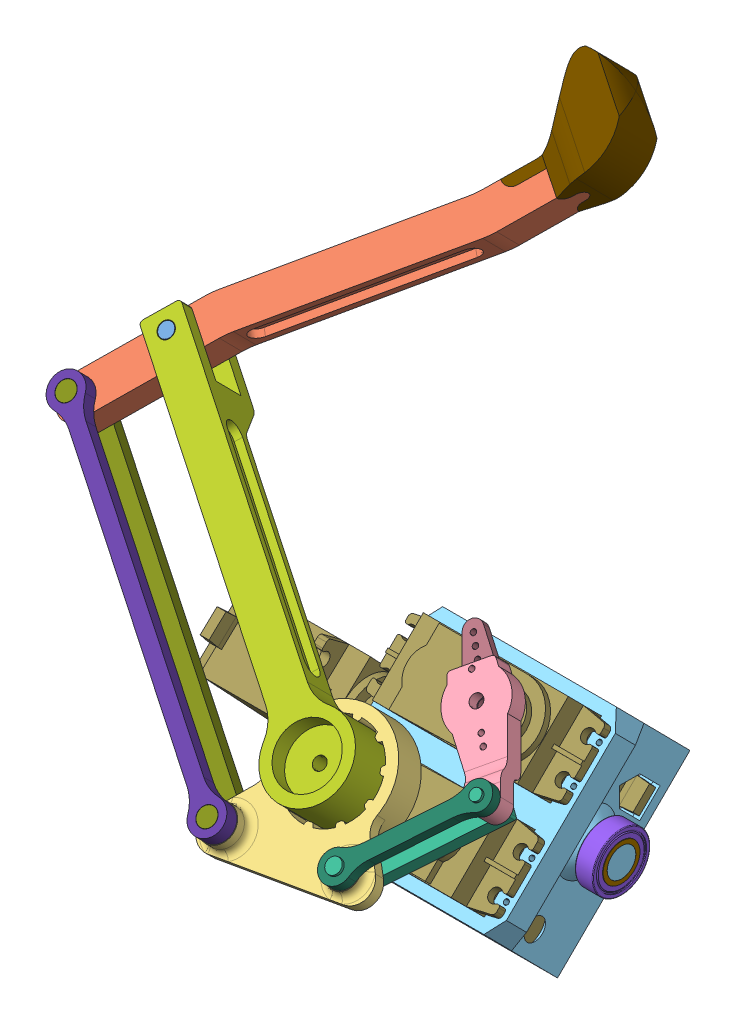
SolidWorks assembly Leg 2, configuration Default. Lengths in mm.
Overall size (147.89 165.46 140.11).
31 component instances, 18 part files, 42 mates.
Components (placement in the parent):
- Dowel-1: Dowel [Default] at (-255.223 372.999 -15.2268) x (0.218857 -0.685853 0.694051) z (0 0.711295 0.702894) size (3.9 3.9 20)
- Lower leg-1: Lower leg [Default] at (-184.6898 434.9539 -55.8705) x (0.812101 -0.41015 0.415052) z (0 -0.711295 -0.702894) size (20 126 9)
- Rotating Piece-1: Rotating Piece [Default] at (-173.9415 332.1367 27.2621) x (0.180878 0.6913 -0.699562) z (0.983506 -0.127138 0.128657) size (44.28 13.7 43.21)
- Servo Arm Mount-1: Servo Arm Mount [Default] at (-152.9415 354.3242 12.3496) x (-0.715783 -0.490847 0.496713) z (0 0.711295 0.702894) size (16.2 34.39 8.1)
- Servo Housing 3-1: Servo Housing 3 [Default] at (-163.4415 323.5657 18.6498) x (1 0 0) z (0 0.711295 0.702894) size (61.5 52 29.25)
- Short Connecting Rod-1: Short Connecting Rod [Default] at (-137.7959 345.0213 22.475) x (-0.625384 -0.54848 0.555035) z (0 -0.711295 -0.702894) size (37.08 4 13)
- Upper Leg-1: Upper Leg [Default] at (-261.8797 379.1638 -7.2384) x (-0.587065 -0.569021 0.575822) z (0 0.711295 0.702894) size (22 116.4 18)
- 688ZZ Bearing Assembly-1: 688ZZ Bearing Assembly [Default] at (-131.6915 320.8602 -2.3002) x (0 0 -1) z (1 0 0) size (17.99 17.98 5)
  - Outer Ring-1: Outer Ring [Default] at origin size (16 16 5)
  - Inner Ring-1: Inner Ring [Default] x (-0.241565 -0.970385 0) z (0 0 1) size (10.6 10.6 5)
  - Cage-1: Cage [Default] x (0.535517 0.844524 0) z (0 0 1) size (13.01 13.06 2.21)
  - 2mm Ball Bearing-1: 2mm Ball Bearing [Default] at (-5.0671 3.2131 0) x (0.050652 0.835774 0.546732) z (0.977207 -0.154478 0.145614) size (2 2 2)
  - 2mm Ball Bearing-2: 2mm Ball Bearing [Default] at (-5.988 -0.3789 0) x (-0.450278 0.705928 0.546732) z (0.881377 0.449412 0.145614) size (2 2 2)
  - 2mm Ball Bearing-3: 2mm Ball Bearing [Default] at (-4.6217 -3.8262 0) x (-0.779216 0.306441 0.546732) z (0.448891 0.881642 0.145614) size (2 2 2)
  - 2mm Ball Bearing-4: 2mm Ball Bearing [Default] at (-1.49 -5.812 0) x (-0.810521 -0.210096 0.546732) z (-0.155056 0.977115 0.145614) size (2 2 2)
  - 2mm Ball Bearing-5: 2mm Ball Bearing [Default] at (2.2108 -5.5778 0) x (-0.532234 -0.646383 0.546732) z (-0.699777 0.699363 0.145614) size (2 2 2)
  - 2mm Ball Bearing-6: 2mm Ball Bearing [Default] at (5.0671 -3.2131 0) x (-0.050652 -0.835774 0.546732) z (-0.977207 0.154478 0.145614) size (2 2 2)
  - 2mm Ball Bearing-7: 2mm Ball Bearing [Default] at (5.988 0.3789 0) x (0.450278 -0.705928 0.546732) z (-0.881377 -0.449412 0.145614) size (2 2 2)
  - 2mm Ball Bearing-8: 2mm Ball Bearing [Default] at (4.6217 3.8262 0) x (0.779216 -0.306441 0.546732) z (-0.448891 -0.881642 0.145614) size (2 2 2)
  - 2mm Ball Bearing-9: 2mm Ball Bearing [Default] at (1.49 5.812 0) x (0.810521 0.210096 0.546732) z (0.155056 -0.977115 0.145614) size (2 2 2)
  - 2mm Ball Bearing-10: 2mm Ball Bearing [Default] at (-2.2108 5.5778 0) x (0.532234 0.646383 0.546732) z (0.699777 -0.699363 0.145614) size (2 2 2)
- MG996R-1: MG996R [Default] at (-163.4415 321.9958 -19.4546) x (-1 0 0) z (0 0.702894 -0.711295) size (54.5 42.75 20)
- MG996R-2: MG996R [Default] at (-163.4415 303.7205 -0.9609) x (1 0 0) z (0 -0.702894 0.711295) size (54.5 42.75 20)
- Double_Blade_Rudder-1: Double_Blade_Rudder [默认] at (-152.9415 354.2531 12.2793) x (-0.715783 -0.490847 0.496713) z (0.698322 -0.50312 0.509133) size (12.2 5.5 38)
- Circle Rudder-2: Circle Rudder [默认] at (-173.9415 335.8354 30.9171) x (0.268347 0.677113 -0.685206) z (-0.963322 0.18862 -0.190874) size (20.8 5.5 20.8)
- Circle Rudder-3: Circle Rudder [默认] at (-190.6915 320.8602 -2.3002) x (0 0.990513 -0.137416) z (0 0.137416 0.990513) size (20.8 5.5 20.8)
- MG996R-3: MG996R [Default] at (-235.7415 313.2801 -9.5667) x (0 -0.728522 -0.685022) z (0 -0.685022 0.728522) size (54.5 42.75 20)
- Short Connecting Rod Alt-1: Short Connecting Rod Alt [Default] at (-158.1737 328.6713 46.5607) x (-0.625384 -0.54848 0.555035) z (-0.780317 0.439579 -0.444832) size (41.18 3 8.1)
- Long Connecting Rod-1: Long Connecting Rod [Default] at (-185.0416 322.3134 45.3121) x (0.80954 -0.412644 0.417576) z (0 -0.711295 -0.702894) size (105.4 5 16)
- Long Connecting Rod Alt-1: Long Connecting Rod Alt [Default] at (-188.5331 327.6128 51.3309) x (0.80954 -0.412644 0.417576) z (-0.587065 -0.569021 0.575821) size (109.5 4 9.1)
- Foot Cap R2-1: Foot Cap R2 [Default] at (-184.6898 434.9539 -55.8705) x (0.812101 -0.41015 0.415052) z (0 -0.711295 -0.702894) size (26.22 31.5 15)
Mates (geometry in assembly coordinates):
- Coincident1: coincident anti-aligned: plane of Servo Housing 3-1 through (-163.4415 260.0708 -66.5893) normal (0 0.702894 -0.711295); plane of MG996R-1 through (-143.1915 340.3956 12.7868) normal (0 -0.702894 0.711295)
- Concentric1: concentric aligned: cylinder of Servo Housing 3-1 through (-138.4415 331.0182 -3.83) axis (0 0.711295 0.702894) radius 0.7; cylinder of MG996R-1 through (-138.4415 338.0245 3.0935) axis (0 0.711295 0.702894) radius 1.7678
- Distance1: distance = 1.85 mm anti-aligned: plane of MG996R-1 through (-138.4415 338.0245 3.0935) normal (0 -0.711295 -0.702894); plane of Servo Housing 3-1 through (-163.4415 321.7874 16.8926) normal (0 0.711295 0.702894)
- Coincident6: coincident aligned: plane of MG996R-1 through (-138.4415 339.8027 4.8507) normal (0 0.711295 0.702894); plane of MG996R-2 through (-188.4415 328.2356 16.556) normal (0 0.711295 0.702894)
- Concentric7: concentric aligned: cylinder of MG996R-1 through (-152.9415 350.341 8.4134) axis (0 0.711295 0.702894) radius 1.5; cylinder of Double_Blade_Rudder-1 through (-152.9415 350.341 8.4134) axis (0 0.711295 0.702894) radius 3
- Concentric8: concentric aligned: cylinder of MG996R-2 through (-173.9415 331.9233 27.0512) axis (0 0.711295 0.702894) radius 1.5; cylinder of Circle Rudder-2 through (-173.9415 331.9233 27.0512) axis (0 0.711295 0.702894) radius 3
- Coincident8: coincident anti-aligned: plane of MG996R-2 through (-173.9415 331.9233 27.0512) normal (0 0.711295 0.702894); plane of Circle Rudder-2 through (-173.9415 331.9233 27.0512) normal (0 -0.711295 -0.702894)
- Coincident9: coincident anti-aligned: plane of MG996R-1 through (-152.9415 350.341 8.4134) normal (0 0.711295 0.702894); plane of Double_Blade_Rudder-1 through (-152.9415 350.341 8.4134) normal (0 -0.711295 -0.702894)
- Coincident10: coincident anti-aligned: plane of Servo Housing 3-1 through (-190.6915 248.8245 -55.2086) normal (-1 0 0); plane of Circle Rudder-3 through (-190.6915 320.8602 -2.3002) normal (1 0 0)
- Concentric9: concentric anti-aligned: cylinder of Servo Housing 3-1 through (-170.6915 320.8602 -2.3002) axis (-1 0 0) radius 4.5; cylinder of Circle Rudder-3 through (-196.1915 320.8602 -2.3002) axis (1 0 0) radius 3
- Concentric10: concentric anti-aligned: cylinder of Servo Arm Mount-1 through (-152.9415 356.4581 14.4583) axis (0 -0.711295 -0.702894) radius 1.7; cylinder of Double_Blade_Rudder-1 through (-152.9415 352.6171 10.6626) axis (0 0.711295 0.702894) radius 1.5
- Coincident11: coincident anti-aligned: plane of Servo Arm Mount-1 through (-152.9415 354.2531 12.2793) normal (0 -0.711295 -0.702894); plane of Double_Blade_Rudder-1 through (-152.9415 354.2531 12.2793) normal (0 0.711295 0.702894)
- Concentric11: concentric aligned: cylinder of Servo Arm Mount-1 through (-145.9582 349.2219 17.3706) axis (0 0.711295 0.702894) radius 0.75; cylinder of Double_Blade_Rudder-1 through (-145.9582 347.5859 15.754) axis (0 0.711295 0.702894) radius 0.75
- Concentric12: concentric anti-aligned: cylinder of Servo Housing 3-1 through (-129.1915 320.8602 -2.3002) axis (-1 0 0) radius 4; cylinder of 688ZZ Bearing Assembly-1/Inner Ring-1 through (-124.9361 320.8602 -2.3002) axis (1 0 0) radius 4
- Coincident12: coincident anti-aligned: plane of Servo Housing 3-1 through (-134.1915 320.8602 -2.3002) normal (1 0 0); plane of 688ZZ Bearing Assembly-1/Inner Ring-1 through (-134.1915 319.6162 -7.2977) normal (-1 0 0)
- Coincident13: coincident anti-aligned: plane of Upper Leg-1 through (-173.9415 335.8354 30.9171) normal (0 -0.711295 -0.702894); plane of Circle Rudder-2 through (-173.9415 335.8354 30.9171) normal (0 0.711295 0.702894)
- Concentric13: concentric anti-aligned: cylinder of Upper Leg-1 through (-173.9415 342.237 37.2431) axis (0 -0.711295 -0.702894) radius 1.7; cylinder of Circle Rudder-2 through (-173.9415 334.1994 29.3004) axis (0 0.711295 0.702894) radius 1.5
- Concentric14: concentric aligned: cylinder of Servo Housing 3-1 through (-188.4415 312.4222 14.9882) axis (0 0.711295 0.702894) radius 0.7; cylinder of MG996R-2 through (-188.4415 319.4285 21.9117) axis (0 0.711295 0.702894) radius 1.7678
- Concentric15: concentric aligned: cylinder of Servo Housing 3-1 through (-188.4415 319.4512 7.8753) axis (0 0.711295 0.702894) radius 0.7; cylinder of MG996R-2 through (-188.4415 326.4574 14.7988) axis (0 0.711295 0.702894) radius 1.7678
- Concentric16: concentric anti-aligned: cylinder of Rotating Piece-1 through (-173.9415 333.5593 28.6678) axis (0 -0.711295 -0.702894) radius 4.35; cylinder of Circle Rudder-2 through (-173.9415 331.9233 27.0512) axis (0 0.711295 0.702894) radius 4.4
- Coincident14: coincident aligned: plane of Rotating Piece-1 through (-156.0716 324.3934 43.3494) normal (0 -0.711295 -0.702894); plane of Servo Arm Mount-1 through (-137.1733 343.3194 24.1972) normal (0 -0.711295 -0.702894)
- Concentric17: concentric aligned: cylinder of Lower leg-1 through (-255.223 377.6224 -10.658) axis (0 0.711295 0.702894) radius 2; cylinder of Upper Leg-1 through (-255.223 374.4216 -13.8211) axis (0 0.711295 0.702894) radius 2.1
- Concentric21: concentric anti-aligned: cylinder of Dowel-1 through (-255.223 387.2249 -1.169) axis (0 -0.711295 -0.702894) radius 1.95; cylinder of Upper Leg-1 through (-255.223 374.4216 -13.8211) axis (0 0.711295 0.702894) radius 2.1
- Coincident15: coincident aligned: plane of Dowel-1 through (-255.223 387.2249 -1.169) normal (0 0.711295 0.702894); plane of Upper Leg-1 through (-261.8797 386.2767 -0.2094) normal (0 0.711295 0.702894)
- Distance2: distance = 0.5 mm anti-aligned: plane of Lower leg-1 through (-184.6898 434.9539 -55.8705) normal (0 0.711295 0.702894); plane of Upper Leg-1 through (-252.4867 392.5359 -12.2341) normal (0 -0.711295 -0.702894)
- Coincident17: coincident anti-aligned: plane of Rotating Piece-1 through (-156.0716 324.3934 43.3494) normal (0 -0.711295 -0.702894); plane of Short Connecting Rod-1 through (-137.7959 345.0213 22.475) normal (0 0.711295 0.702894)
- Concentric27: concentric aligned: cylinder of Circle Rudder-3 through (-196.1915 320.8602 -2.3002) axis (1 0 0) radius 3; cylinder of MG996R-3 through (-195.9915 320.8602 -2.3002) axis (1 0 0) radius 1.5
- Coincident18: coincident anti-aligned: plane of Circle Rudder-3 through (-192.9915 320.8602 -2.3002) normal (-1 0 0); plane of MG996R-3 through (-192.9915 320.8602 -2.3002) normal (1 0 0)
- Concentric28: concentric anti-aligned: cylinder of Servo Arm Mount-1 through (-137.1733 341.3278 22.2291) axis (0 0.711295 0.702894) radius 1.7; cylinder of Short Connecting Rod-1 through (-137.1733 349.7211 30.5233) axis (0 -0.711295 -0.702894) radius 1.5
- Concentric29: concentric aligned: cylinder of Rotating Piece-1 through (-158.1737 327.1776 45.0846) axis (0 -0.711295 -0.702894) radius 2.2; cylinder of Short Connecting Rod-1 through (-158.1737 331.3031 49.1614) axis (0 -0.711295 -0.702894) radius 2
- Concentric30: concentric aligned: cylinder of Short Connecting Rod-1 through (-158.1737 331.3031 49.1614) axis (0 -0.711295 -0.702894) radius 2; cylinder of Short Connecting Rod Alt-1 through (-158.1737 330.8052 48.6694) axis (0 -0.711295 -0.702894) radius 2.05
- Coincident20: coincident anti-aligned: plane of Rotating Piece-1 through (-173.9415 340.032 35.0642) normal (0 0.711295 0.702894); plane of Short Connecting Rod Alt-1 through (-158.1737 328.6713 46.5607) normal (0 -0.711295 -0.702894)
- Concentric33: concentric aligned: cylinder of Short Connecting Rod-1 through (-137.1733 349.7211 30.5233) axis (0 -0.711295 -0.702894) radius 1.5; cylinder of Short Connecting Rod Alt-1 through (-137.1733 349.2232 30.0313) axis (0 -0.711295 -0.702894) radius 1.55
- Concentric35: concentric anti-aligned: cylinder of Rotating Piece-1 through (-188.5331 324.2697 48.0273) axis (0 -0.711295 -0.702894) radius 2.7; cylinder of Long Connecting Rod-1 through (-188.5331 319.0772 42.8961) axis (0 0.711295 0.702894) radius 2.5
- Coincident21: coincident anti-aligned: plane of Lower leg-1 through (-184.6898 428.5523 -62.1966) normal (0 -0.711295 -0.702894); plane of Long Connecting Rod-1 through (-185.0416 322.3134 45.3121) normal (0 0.711295 0.702894)
- Concentric36: concentric aligned: cylinder of Lower leg-1 through (-269.8109 363.3519 3.7831) axis (0 0.711295 0.702894) radius 2.6; cylinder of Long Connecting Rod-1 through (-269.8109 360.5067 0.9715) axis (0 0.711295 0.702894) radius 2.5
- Concentric37: concentric anti-aligned: cylinder of Long Connecting Rod-1 through (-188.5331 319.0772 42.8961) axis (0 0.711295 0.702894) radius 2.5; cylinder of Long Connecting Rod Alt-1 through (-188.5331 330.458 54.1424) axis (0 -0.711295 -0.702894) radius 2.55
- Coincident22: coincident anti-aligned: plane of Lower leg-1 through (-276.789 368.2389 10.2192) normal (0 0.711295 0.702894); plane of Long Connecting Rod Alt-1 through (-188.5331 327.6128 51.3309) normal (0 -0.711295 -0.702894)
- Concentric38: concentric anti-aligned: cylinder of Long Connecting Rod-1 through (-269.8109 360.5067 0.9715) axis (0 0.711295 0.702894) radius 2.5; cylinder of Long Connecting Rod Alt-1 through (-269.8109 371.8874 12.2178) axis (0 -0.711295 -0.702894) radius 2.55
- Concentric39: concentric aligned: cylinder of Lower leg-1 through (-201.296 421.5312 -48.6895) axis (-0.812101 0.41015 -0.415052) radius 2; cylinder of Foot Cap R2-1 through (-201.296 421.5312 -48.6895) axis (-0.812101 0.41015 -0.415052) radius 2
- Concentric40: concentric aligned: cylinder of Lower leg-1 through (-195.1691 427.5336 -54.746) axis (0.812101 -0.41015 0.415052) radius 2; cylinder of Foot Cap R2-1 through (-195.1691 427.5336 -54.746) axis (0.812101 -0.41015 0.415052) radius 2
- Concentric41: concentric aligned: cylinder of Lower leg-1 through (-192.2515 433.5798 -54.4799) axis (0 -0.711295 -0.702894) radius 2; cylinder of Foot Cap R2-1 through (-192.2515 433.5798 -54.4799) axis (0 -0.711295 -0.702894) radius 2
